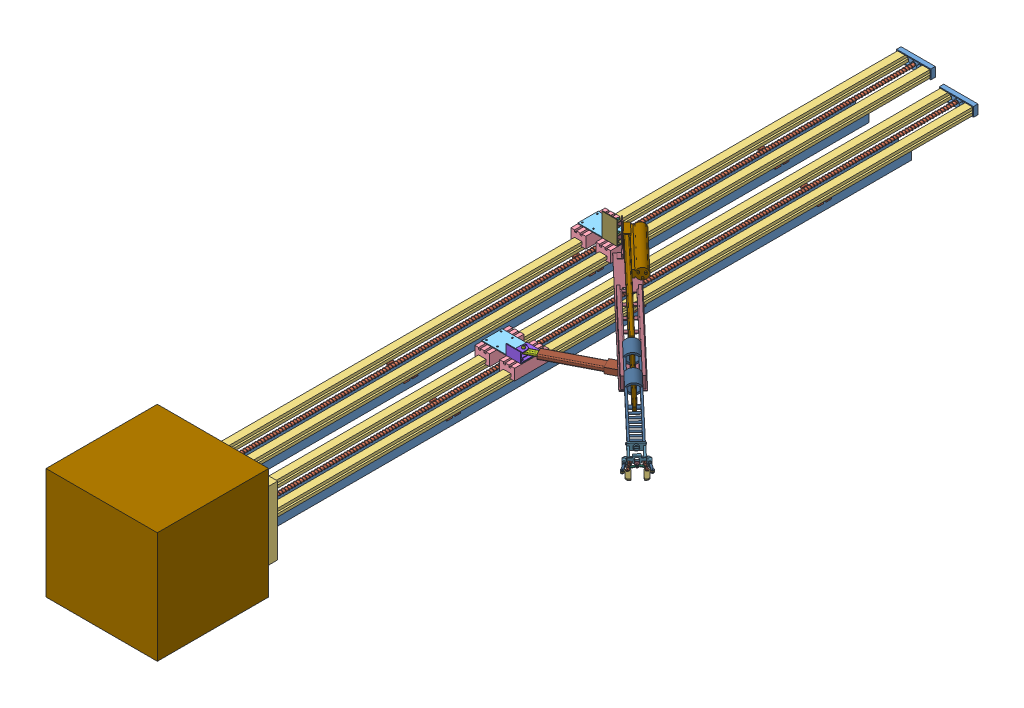
SolidWorks assembly obtox-LIBERO, configuration Default. Lengths in mm.
Overall size (778.48 300 2255.5).
74 component instances, 34 part files, 123 mates.
Components (placement in the parent):
- tapadera de riel-1: tapadera de riel [Default] at (-0.4886 54.6546 45.8092) size (92.3 25.3 12)
- husillo 1900mm-1: husillo 1900mm [Default] at (45.6614 67.3046 1945.8092) x (-0.808521 -0.588468 0) z (0.588468 -0.808521 0) size (10.19 1900.05 10.19)
- tapadera de riel-2: tapadera de riel [Default] at (-115.4886 84.6546 45.8092) size (92.3 25.3 12)
- husillo 1900mm-2: husillo 1900mm [Default] at (-69.3386 97.3046 1945.8092) x (0.990967 -0.134107 0) z (0.134107 0.990967 0) size (10.19 1900.05 10.19)
- guia lineal 2000mm-6: guia lineal 2000mm [Default] at (89.3114 57.1546 1023.3092) x (0 1 0) z (-1 0 0) size (20.3 1950 20.3)
- guia lineal 2000mm-7: guia lineal 2000mm [Default] at (22.3114 57.1546 1023.3092) x (0 1 0) z (-1 0 0) size (20.3 1950 20.3)
- guia lineal 2000mm-8: guia lineal 2000mm [Default] at (-25.6886 87.1546 1023.3092) x (0 1 0) z (-1 0 0) size (20.3 1950 20.3)
- guia lineal 2000mm-9: guia lineal 2000mm [Default] at (-92.6886 87.1546 1023.3092) x (0 1 0) z (-1 0 0) size (20.3 1950 20.3)
- brazo1-1: brazo1 [Default] at (-20.1441 63.0474 912.1315) x (-1 0 0) z (0 0 -1) size (107 44.63 92.2)
  - cojinete-1: cojinete [Default] at (82.6945 46.8572 -15.9576) size (40 30 92.2)
  - cojinete-2: cojinete [Default] at (15.6945 46.8572 -15.9576) size (40 30 92.2)
  - base brazo-1: base brazo [Default] at (49.1945 63.8572 30.1424) x (1 0 0) z (0 -1 0) size (107 55 40.6)
  - tuerca trapezoidal 8-1: tuerca trapezoidal 8 [Default] at (49.1945 34.2572 38.1424) x (0.866025 0.5 0) z (0.5 -0.866025 0) size (22 14.94 22)
- brazo1-2: brazo1 [Default] at (-3.5331 33.0474 1225.8074) size (107 44.63 92.2)
  - cojinete-1: cojinete [Default] at (82.6945 46.8572 -15.9576) size (40 30 92.2)
  - cojinete-2: cojinete [Default] at (15.6945 46.8572 -15.9576) size (40 30 92.2)
  - base brazo-1: base brazo [Default] at (49.1945 63.8572 30.1424) x (1 0 0) z (0 -1 0) size (107 55 40.6)
  - tuerca trapezoidal 8-1: tuerca trapezoidal 8 [Default] at (49.1945 34.2572 38.1424) x (0.866025 0.5 0) z (0.5 -0.866025 0) size (22 14.94 22)
- actuador 1-B-1: actuador 1-B [Default] at (146.7453 121.4046 1238.9625) x (-0.888465 0 0.458945) z (0 -1 0) size (165.5 12 10)
- base actuador 1-2: base actuador 1 [Default] at (59.1614 96.9046 1283.4497) size (40 27 57)
- actuador 1-C-3: actuador 1-C [Default] at (-3.3143 159.4046 907.6709) x (0.725073 0 0.688672) z (0.688672 0 -0.725073) size (384.5 50 48.5)
- deslizante1-1: deslizante1 [Default] at (415.9571 159.4046 1295.5495) x (0.725073 0 0.688672) z (-0.688672 0 0.725073) size (334.5 28.83 40)
- actuador 1-A-5: actuador 1-A [Default] at (253.4869 121.4046 1183.8241) x (-0.888465 0 0.458945) z (0 -1 0) size (184.5 30 15)
- base actuador 3-2: base actuador 3 [Default] at (-55.8386 126.9046 909.4892) size (40 62 29.5)
- Ensamblaje1^obtox-LIBERO-1: Ensamblaje1^obtox-LIBERO [Default] at (400.9916 0 -830.6547) x (0.974334 0 0.225105) z (-0.225105 0 0.974334) size (467.29 65.5 306.35) (virtual)
  - base actuador 2-1: base actuador 2 [Default] at (-2.6233 159.4046 1784.7219) x (0.861487 0 0.507779) z (-0.507779 0 0.861487) size (510 65.5 55)
- servo MG995-1: servo MG995 [Default] at (-79.1886 127.7046 1998.1092) x (1 0 0) z (0 1 0) size (21.2 45.8 54)
- perno2-2: perno2 [Default] at (-21.8386 134.1942 902.4892) x (0.900304 0 -0.435263) z (0 1 0) size (6 6 20)
- perno2-3: perno2 [Default] at (-21.8386 185.6169 902.4892) x (-0.763428 0 0.645893) z (0 -1 0) size (6 6 20)
- perno-3: perno [Default] at (89.6614 124.3697 1268.4497) x (0.731791 0 0.681529) z (0 -1 0) size (8 8 20)
- servo MG995-3: servo MG995 [Default] at (35.8114 97.7046 1998.1092) x (1 0 0) z (0 1 0) size (21.2 45.8 54)
- cople flefible 6x8-2: cople flefible 6x8 [Default] at (45.6614 67.3046 1953.8092) x (0.367009 -0.930217 0) z (0.930217 0.367009 0) size (17.8 25 17.8)
- actuador 1-D-1: actuador 1-D [Default] at (374.5362 159.4046 1245.8643) x (0.725073 0 0.688672) z (-0.688672 0 0.725073) size (368 12 10)
- soporte perfil 40x40x4 mm-2: soporte perfil 40x40x4 mm [Default] at (-49.3386 82.1546 1998.3092) x (-1 0 0) z (0 0 -1) size (40 40 1800)
- soporte L para base-1: soporte L para base [Default] at (-61.8386 17.1546 1998.3092) x (0 1 0) z (0 0 1) size (25 15 25)
- soporte L para base-2: soporte L para base [Default] at (-114.3386 54.6546 1998.3092) size (25 15 25)
- soporte L para base-3: soporte L para base [Default] at (-24.3386 69.6546 1998.3092) x (-1 0 0) z (0 0 1) size (25 15 25)
- soporte L para base-4: soporte L para base [Default] at (-89.3386 62.1546 1438.8092) x (0 1 0) z (1 0 0) size (25 15 25)
- soporte perfil 40x40x4 mm-3: soporte perfil 40x40x4 mm [Default] at (65.6614 52.1546 1998.3092) x (-1 0 0) z (0 0 -1) size (40 40 1800)
- soporte L para base-5: soporte L para base [Default] at (0.6614 24.6546 1998.3092) size (25 15 25)
- soporte L para base-7: soporte L para base [Default] at (53.1614 -12.8454 1998.3092) x (0 1 0) z (0 0 1) size (25 15 25)
- soporte L para base-8: soporte L para base [Default] at (90.6614 39.6546 1998.3092) x (-1 0 0) z (0 0 1) size (25 15 25)
- tapadera de base-1: tapadera de base [Default] at (112.6614 40.3046 1998.3092) x (-1 0 0) z (0 0 -1) size (249 184 44.5)
- tornillo-2: tornillo [Default] at (275.4764 116.9046 1172.4652) x (0.394703 0 -0.918809) z (0 1 0) size (10 11.55 18)
- buje-2: buje [Default] at (275.4764 121.9046 1172.4652) x (0.303677 0 -0.952775) z (0 1 0) size (8 8 10)
- tuerca-2: tuerca [Default] at (275.4764 108.4046 1172.4652) x (-0.848097 0 -0.529841) z (0 1 0) size (10 11.55 5.31)
- cople flefible 6x8-3: cople flefible 6x8 [Default] at (-69.3386 97.3046 1953.8092) x (0.981829 -0.189768 0) z (0.189768 0.981829 0) size (17.8 25 17.8)
- brida para  husillo-3: brida para  husillo [Default] at (-69.3386 97.3046 1928.8092) x (0 -1 0) z (0 0 1) size (45 30 25)
- brida para  husillo-4: brida para  husillo [Default] at (45.6614 67.3046 1928.8092) x (0 -1 0) z (0 0 1) size (45 30 25)
- soporte L para base-9: soporte L para base [Default] at (-49.3386 62.1546 1453.8092) x (0 1 0) z (-1 0 0) size (25 15 25)
- soporte L para base-10: soporte L para base [Default] at (-89.3386 62.1546 938.8092) x (0 1 0) z (1 0 0) size (25 15 25)
- soporte L para base-11: soporte L para base [Default] at (-89.3386 62.1546 438.8092) x (0 1 0) z (1 0 0) size (25 15 25)
- soporte L para base-12: soporte L para base [Default] at (-49.3386 62.1546 953.8092) x (0 1 0) z (-1 0 0) size (25 15 25)
- soporte L para base-13: soporte L para base [Default] at (-49.3386 62.1546 453.8092) x (0 1 0) z (-1 0 0) size (25 15 25)
- soporte L para base-14: soporte L para base [Default] at (0.6614 57.1546 1453.8092) x (1 0 0) z (0 1 0) size (25 15 25)
- soporte L para base-15: soporte L para base [Default] at (65.6614 32.1546 1453.8092) x (0 1 0) z (-1 0 0) size (25 15 25)
- soporte L para base-16: soporte L para base [Default] at (65.6614 32.1546 953.8092) x (0 1 0) z (-1 0 0) size (25 15 25)
- soporte L para base-17: soporte L para base [Default] at (65.6614 32.1546 453.8092) x (0 1 0) z (-1 0 0) size (25 15 25)
- soporte L para base-18: soporte L para base [Default] at (0.6614 57.1546 953.8092) x (1 0 0) z (0 1 0) size (25 15 25)
- soporte L para base-19: soporte L para base [Default] at (0.6614 57.1546 453.8092) x (1 0 0) z (0 1 0) size (25 15 25)
- base-3: base [Default] at (45.6614 67.3046 2001.3092) x (-1 0 0) z (0 0 -1) size (249 184 15)
- soporte-1: soporte [Default] at (-14.1555 78.9736 2001.3092) size (300 300 300)
- pinza-1: pinza [Default] at (541.5071 178.6079 1428.4206) x (0.683645 0.000003 0.729815) z (0.000007 -1 -0.000002) size (126.59 67.98 17)
  - eslabon1-1: eslabon1 [Default] at (16.7384 15.8668 19.3533) x (0.993867 0.110585 0.000003) z (-0.000003 0.000007 1) size (32.5 7.5 7.18)
  - eslabon3-1: eslabon3 [Default] at (16.1548 5.8838 19.3533) x (0.993867 0.110585 0.000003) z (-0.000003 0.000007 1) size (32.5 7.5 7.18)
  - eslabon1-2: eslabon1 [Default] at (13.6225 -37.4322 19.3536) x (0.97421 -0.225641 0.000005) z (-0.000003 0.000007 1) size (32.5 7.5 7.18)
  - clamp-4: clamp [Default] at (29.1618 17.2491 19.4033) x (0.998295 -0.058362 0.000004) z (-0.000003 0.000007 1) size (32.2 19.9 3.4)
  - embolo-1: embolo [Default] at (8.4631 -10.39 23.0534) x (0.058362 0.998295 -0.000007) z (0.000003 -0.000007 -1) size (10 10.75 10)
  - agarradera-amp-1: agarradera-amp [Default] at (-58.5297 18.3293 -31.8016) x (-0.058362 -0.998295 0.000007) z (-0.000003 0.000007 1) size (56.98 73.9 17)
  - clamp-5: clamp [Default] at (25.8001 -40.2528 19.4037) x (0.998295 -0.058362 0.000004) z (0.000003 -0.000007 -1) size (32.2 19.9 3.4)
  - eslabon3-4: eslabon3 [Default] at (14.2061 -27.4493 19.3536) x (0.97421 -0.225641 0.000005) z (0.000003 -0.000007 -1) size (32.5 7.5 7.18)
  - eslabon2-1: eslabon2 [Default] at (8.4631 -10.39 19.5534) x (0.427317 0.904102 -0.000005) z (-0.000003 0.000007 1) size (25.2 7.2 1.5)
  - eslabon2-2: eslabon2 [Default] at (8.4631 -10.39 18.0534) x (0.319055 -0.947736 0.000008) z (-0.000003 0.000007 1) size (25.2 7.2 1.5)
- martillo-2: martillo [Default] at (593.6439 324.9515 1443.0766) x (0.725073 0 0.688672) z (-0.688672 0 0.725073) size (125.98 327.7 54.17) (hidden)
Mates (geometry in assembly coordinates):
- Concéntrica2: concentric aligned: circle of tapadera de riel-1; circle of husillo-1
- Coincidente9: coincident aligned: plane of tapadera de riel-1 through (-0.4886 54.6546 45.8092) normal (0 0 -1); plane of husillo 1900mm-1 through (45.6614 67.3046 45.8092) normal (0 0 -1)
- Coincidente40: coincident: plane of tapadera de riel-1 through (-0.4886 54.6546 45.8092) normal (0 0 -1); plane of tapadera de riel-2 through (-115.4886 84.6546 45.8092) normal (0 0 -1)
- Coincidente45: coincident anti-aligned: plane of tapadera de riel-1 through (-0.4886 57.1546 57.8092) normal (0 1 0); plane of guia lineal 2000mm-6 through (69.0114 57.1546 48.3092) normal (0 -1 0)
- Coincidente46: coincident anti-aligned: plane of tapadera de riel-1 through (89.3114 54.6546 57.8092) normal (-1 0 0); plane of guia lineal 2000mm-6 through (89.3114 57.1546 48.3092) normal (1 0 0)
- Coincidente47: coincident anti-aligned: plane of tapadera de riel-1 through (-0.4886 54.6546 48.3092) normal (0 0 1); plane of guia lineal 2000mm-6 through (89.3114 57.1546 48.3092) normal (0 0 -1)
- Coincidente53: coincident anti-aligned: plane of tapadera de riel-2 through (-115.4886 84.6546 48.3092) normal (0 0 1); plane of guia lineal 2000mm-8 through (-25.6886 87.1546 48.3092) normal (0 0 -1)
- Coincidente59: coincident anti-aligned: plane of tapadera de riel-2 through (-115.4886 87.1546 57.8092) normal (0 1 0); plane of guia lineal 2000mm-9 through (-112.9886 87.1546 48.3092) normal (0 -1 0)
- Coincidente60: coincident anti-aligned: plane of tapadera de riel-2 through (-112.9886 84.6546 57.8092) normal (1 0 0); plane of guia lineal 2000mm-9 through (-112.9886 94.8046 48.3092) normal (-1 0 0)
- Concéntrica4: concentric anti-aligned: circle of tapadera de riel-2; circle of brazo1-1/tuerca trapezoidal-1
- Paralelo1: parallel aligned: plane of guia lineal 2000mm-8 through (-25.6886 107.4546 48.3092) normal (0 1 0); plane of brazo1-1/cojinete-2 through (-15.8386 124.9046 835.8892) normal (0 1 0)
- Concéntrica5: concentric aligned: circle of husillo-1; circle of brazo1-2/tuerca trapezoidal-1
- Paralelo2: parallel aligned: plane of guia lineal 2000mm-6 through (89.3114 77.4546 48.3092) normal (0 1 0); plane of brazo1-2/base brazo-1 through (45.6614 96.9046 1255.9497) normal (0 1 0)
- Concéntrica6: concentric anti-aligned: circle of brazo1-2/base brazo-1; circle of base actuador 1-1
- Concéntrica7: concentric anti-aligned: circle of brazo1-2/base brazo-1; circle of base actuador 1-1
- Concéntrica8: concentric anti-aligned: circle of brazo1-2/base brazo-1; circle of base actuador 1-1
- Coincidente61: coincident anti-aligned: plane of brazo1-2/base brazo-1 through (45.6614 96.9046 1255.9497) normal (0 1 0); plane of base actuador 1-2 through (59.1614 96.9046 1283.4497) normal (0 -1 0)
- Concéntrica9: concentric anti-aligned: circle of actuador 1-B-1; circle of base actuador 1-1
- Coincidente64: coincident anti-aligned: plane of actuador 1-B-1 through (146.7453 118.9046 1238.9625) normal (0 1 0); plane of base actuador 1-2 through (89.6614 118.9046 1268.4497) normal (0 -1 0)
- Paralelo4: parallel aligned: plane of tapadera de riel-2 through (-115.4886 109.9546 57.8092) normal (0 1 0); plane of actuador 1-C-3 through (-6.5793 174.4046 883.8822) normal (0 1 0)
- Paralelo5: parallel aligned: plane of actuador 1-C-3 through (-6.5793 174.4046 883.8822) normal (0 1 0); plane of deslizante1-1 through (428.0088 163.9046 1282.8607) normal (0 1 0)
- Concéntrica16: concentric anti-aligned: circle of brazo1-1/base brazo-1; circle of base actuador 3-2
- Concéntrica17: concentric anti-aligned: circle of brazo1-1/base brazo-1; circle of base actuador 3-2
- Coincidente83: coincident anti-aligned: plane of brazo1-1/base brazo-1 through (-69.3386 126.9046 881.9892) normal (0 1 0); plane of base actuador 3-2 through (-55.8386 126.9046 909.4892) normal (0 -1 0)
- Concéntrica31: concentric anti-aligned: circle of perno2-2; circle of base actuador 3-2
- Concéntrica32: concentric anti-aligned: circle of base actuador 3-2; circle of perno2-3
- Concéntrica34: concentric anti-aligned: circle of base actuador 1-2; circle of perno-3
- Coincidente91: coincident aligned: plane of servo MG995-1 through (-73.9886 83.6546 1965.7092) normal (0 0 -1); plane of servo MG995-3 through (41.0114 101.7546 1965.7092) normal (0 0 -1)
- Concéntrica37: concentric anti-aligned: circle of servo MG995-3; circle of cople-2
- Coincidente96: coincident anti-aligned: plane of actuador 1-C-3 through (20.4486 165.4046 917.1387) normal (0 -1 0); plane of actuador 1-D-1 through (404.9005 165.4046 1291.9438) normal (0 1 0)
- Coincidente97: coincident anti-aligned: plane of actuador 1-C-3 through (22.5146 162.4046 914.9635) normal (-0.688672 0 0.725073); plane of actuador 1-D-1 through (372.8145 159.4046 1247.677) normal (0.688672 0 -0.725073)
- Concéntrica40: concentric anti-aligned: cylinder of deslizante1-1 through (407.3487 159.4046 1304.6129) axis (0.688672 0 -0.725073) radius 4.5; circle of actuador 1-D-1
- Coincidente101: coincident anti-aligned: plane of soporte perfil 40x40x4 mm-2 through (-89.3386 42.1546 198.3092) normal (0 -1 0); plane of soporte L para base-1 through (-76.8386 42.1546 1996.3092) normal (0 1 0)
- Concéntrica41: concentric aligned: circle of soporte perfil 40x40x4 mm-2; circle of soporte L para base-1
- Concéntrica42: concentric anti-aligned: circle of soporte perfil 40x40x4 mm-2; circle of soporte L para base-2
- Coincidente102: coincident anti-aligned: plane of soporte perfil 40x40x4 mm-2 through (-89.3386 82.1546 198.3092) normal (-1 0 0); plane of soporte L para base-2 through (-89.3386 69.6546 1996.3092) normal (1 0 0)
- Concéntrica43: concentric aligned: circle of soporte perfil 40x40x4 mm-2; circle of soporte L para base-3
- Coincidente104: coincident anti-aligned: plane of soporte perfil 40x40x4 mm-2 through (-49.3386 42.1546 198.3092) normal (1 0 0); plane of soporte L para base-3 through (-49.3386 54.6546 1996.3092) normal (-1 0 0)
- Coincidente106: coincident anti-aligned: plane of soporte perfil 40x40x4 mm-2 through (-89.3386 82.1546 198.3092) normal (-1 0 0); plane of soporte L para base-4 through (-89.3386 62.1546 1453.8092) normal (1 0 0)
- Coincidente108: coincident anti-aligned: plane of guia lineal 2000mm-9 through (-112.9886 87.1546 48.3092) normal (0 -1 0); plane of soporte L para base-4 through (-91.3386 87.1546 1453.8092) normal (0 1 0)
- Concéntrica45: concentric aligned: circle of husillo 1900mm-1; circle of cople flefible 6x8-2
- Distancia1: distance = 3.35 mm anti-aligned: plane of soporte perfil 40x40x4 mm-2 through (-49.3386 42.1546 198.3092) normal (1 0 0); plane of guia lineal 2000mm-8 through (-45.9886 94.8046 48.3092) normal (-1 0 0)
- Distancia2: distance = 3.35 mm anti-aligned: plane of soporte perfil 40x40x4 mm-3 through (25.6614 52.1546 198.3092) normal (-1 0 0); plane of guia lineal 2000mm-7 through (22.3114 57.1546 48.3092) normal (1 0 0)
- Concéntrica48: concentric anti-aligned: circle of soporte perfil 40x40x4 mm-3; circle of soporte L para base-5
- Concéntrica51: concentric aligned: circle of soporte perfil 40x40x4 mm-3; circle of soporte L para base-8
- Coincidente116: coincident anti-aligned: plane of soporte perfil 40x40x4 mm-3 through (65.6614 12.1546 198.3092) normal (1 0 0); plane of soporte L para base-8 through (65.6614 24.6546 1996.3092) normal (-1 0 0)
- Distancia3: distance = 20 mm aligned: plane of soporte perfil 40x40x4 mm-2 through (-89.3386 42.1546 198.3092) normal (0 -1 0); plane of soporte L para base-4 through (-92.3386 62.1546 1453.8092) normal (0 -1 0)
- Coincidente118: coincident anti-aligned: plane of soporte perfil 40x40x4 mm-3 through (25.6614 12.1546 198.3092) normal (0 -1 0); plane of soporte L para base-7 through (38.1614 12.1546 1996.3092) normal (0 1 0)
- Concéntrica59: concentric aligned: circle of buje-2; circle of tuerca-2
- Tornillo3: screw = 1 mm aligned: cylinder of husillo 1900mm-1 through (45.6614 67.3046 45.8092) axis (0 0 1) radius 4; cylinder of brazo1-2/tuerca trapezoidal 8-1 through (45.6614 67.3046 1250.4497) axis (0 0 1) radius 4.5
- Coincidente126: coincident anti-aligned: plane of cople flefible 6x8-2 through (48.9278 59.0257 1953.8092) normal (0 0 1); plane of tapadera de base-1 through (112.6614 40.3046 1953.8092) normal (0 0 -1)
- Concéntrica61: concentric anti-aligned: circle of tapadera de base-1; circle of cople flefible 6x8-3
- Coincidente127: coincident aligned: plane of cople flefible 6x8-2 through (45.6614 67.3046 1928.8092) normal (0 0 -1); plane of cople flefible 6x8-3 through (-69.3386 97.3046 1928.8092) normal (0 0 -1)
- Concéntrica62: concentric aligned: circle of cople flefible 6x8-3; circle of brida para  husillo-3
- Paralelo7: parallel anti-aligned: plane of tapadera de base-1 through (-136.3386 40.3046 1953.8092) normal (-1 0 0); plane of brida para  husillo-3 through (-54.3386 109.8046 1953.8092) normal (1 0 0)
- Paralelo8: parallel aligned: plane of servo MG995-1 through (-79.1886 127.7046 1998.1092) normal (-1 0 0); plane of brida para  husillo-3 through (-84.3386 119.8046 1953.8092) normal (-1 0 0)
- Paralelo9: parallel aligned: plane of servo MG995-1 through (-79.1886 127.7046 1998.1092) normal (-1 0 0); plane of servo MG995-3 through (35.8114 97.7046 1998.1092) normal (-1 0 0)
- Coincidente129: coincident anti-aligned: plane of tapadera de base-1 through (112.6614 40.3046 1953.8092) normal (0 0 -1); plane of brida para  husillo-3 through (-69.3386 97.3046 1953.8092) normal (0 0 1)
- Concéntrica63: concentric aligned: circle of cople flefible 6x8-2; circle of brida para  husillo-4
- Coincidente130: coincident aligned: plane of brida para  husillo-3 through (-69.3386 97.3046 1928.8092) normal (0 0 -1); plane of brida para  husillo-4 through (45.6614 67.3046 1928.8092) normal (0 0 -1)
- Paralelo10: parallel aligned: plane of brida para  husillo-3 through (-84.3386 119.8046 1953.8092) normal (-1 0 0); plane of brida para  husillo-4 through (30.6614 89.8046 1953.8092) normal (-1 0 0)
- Distancia5: distance = 500 mm anti-aligned: plane of soporte L para base-4 through (-91.3386 85.1546 1453.8092) normal (0 0 1); plane of tapadera de base-1 through (112.6614 40.3046 1953.8092) normal (0 0 -1)
- Coincidente131: coincident anti-aligned: plane of soporte perfil 40x40x4 mm-2 through (-49.3386 42.1546 198.3092) normal (1 0 0); plane of soporte L para base-9 through (-49.3386 62.1546 1438.8092) normal (-1 0 0)
- Coincidente132: coincident aligned: plane of soporte L para base-4 through (-91.3386 85.1546 1438.8092) normal (0 0 -1); plane of soporte L para base-9 through (-47.3386 85.1546 1438.8092) normal (0 0 -1)
- Coincidente133: coincident aligned: plane of soporte L para base-4 through (-92.3386 62.1546 1453.8092) normal (0 -1 0); plane of soporte L para base-9 through (-46.3386 62.1546 1438.8092) normal (0 -1 0)
- Coincidente134: coincident aligned: plane of soporte L para base-9 through (-47.3386 85.1546 1438.8092) normal (0 0 -1); plane of soporte L para base-14 through (23.6614 55.1546 1438.8092) normal (0 0 -1)
- Coincidente135: coincident anti-aligned: plane of soporte perfil 40x40x4 mm-3 through (25.6614 52.1546 198.3092) normal (-1 0 0); plane of soporte L para base-14 through (25.6614 55.1546 1438.8092) normal (1 0 0)
- Coincidente136: coincident anti-aligned: plane of guia lineal 2000mm-7 through (2.0114 57.1546 48.3092) normal (0 -1 0); plane of soporte L para base-14 through (0.6614 57.1546 1438.8092) normal (0 1 0)
- Coincidente137: coincident anti-aligned: plane of soporte perfil 40x40x4 mm-3 through (65.6614 12.1546 198.3092) normal (1 0 0); plane of soporte L para base-15 through (65.6614 32.1546 1438.8092) normal (-1 0 0)
- Coincidente138: coincident anti-aligned: plane of guia lineal 2000mm-6 through (69.0114 57.1546 48.3092) normal (0 -1 0); plane of soporte L para base-15 through (67.6614 57.1546 1438.8092) normal (0 1 0)
- Coincidente139: coincident aligned: plane of soporte L para base-14 through (23.6614 55.1546 1438.8092) normal (0 0 -1); plane of soporte L para base-15 through (67.6614 55.1546 1438.8092) normal (0 0 -1)
- Coincidente140: coincident anti-aligned: plane of actuador 1-C-3; plane of actuador 1-D-1
- Concéntrica64: concentric aligned: circle of servo MG995-1; circle of cople flefible 6x8-3
- Coincidente141: coincident anti-aligned: plane of servo MG995-1 through (-69.3386 97.3046 1955.8092) normal (0 0 -1); plane of tapadera de base-1 through (112.6614 40.3046 1955.8092) normal (0 0 1)
- Concéntrica66: concentric anti-aligned: circle of tapadera de base-1; circle of brida para  husillo-4
- Coincidente142: coincident aligned: plane of tapadera de base-1 through (-136.3386 40.3046 1953.8092) normal (-1 0 0); plane of base-3 through (-136.3386 70.3046 1998.3092) normal (-1 0 0)
- Coincidente143: coincident aligned: plane of tapadera de base-1 through (112.6614 164.3046 2254.4361) normal (0 1 0); plane of base-3 through (112.6614 164.3046 2257.4361) normal (0 1 0)
- Coincidente144: coincident anti-aligned: plane of soporte L para base-1 through (-76.8386 17.1546 1998.3092) normal (0 0 1); plane of base-3 through (-69.3386 97.3046 1998.3092) normal (0 0 -1)
- Coincidente145: coincident anti-aligned: plane of tapadera de base-1 through (112.6614 40.3046 1998.3092) normal (0 0 1); plane of base-3 through (-69.3386 97.3046 1998.3092) normal (0 0 -1)
- Coincidente146: coincident anti-aligned: plane of tapadera de riel-2 through (-115.4886 107.4546 57.8092) normal (0 -1 0); plane of guia lineal 2000mm-8 through (-25.6886 107.4546 48.3092) normal (0 1 0)
- Coincidente147: coincident anti-aligned: plane of tapadera de riel-2 through (-25.6886 84.6546 57.8092) normal (-1 0 0); plane of guia lineal 2000mm-8 through (-25.6886 87.1546 48.3092) normal (1 0 0)
- Distancia8: distance = 3.35 mm anti-aligned: plane of guia lineal 2000mm-6 through (69.0114 64.8046 48.3092) normal (-1 0 0); plane of soporte perfil 40x40x4 mm-3 through (65.6614 12.1546 198.3092) normal (1 0 0)
- Coincidente149: coincident anti-aligned: plane of soporte L para base-7 through (38.1614 -12.8454 1998.3092) normal (0 0 1); plane of base-3 through (-69.3386 97.3046 1998.3092) normal (0 0 -1)
- Coincidente150: coincident aligned: circle of soporte L para base-5; circle of base-3
- Coincidente152: coincident anti-aligned: plane of soporte L para base-8 through (90.6614 24.6546 1998.3092) normal (0 0 1); plane of base-3 through (-69.3386 97.3046 1998.3092) normal (0 0 -1)
- Concéntrica67: concentric aligned: circle of soporte perfil 40x40x4 mm-3; circle of soporte L para base-7
- Coincidente153: coincident anti-aligned: plane of soporte L para base-3 through (-24.3386 54.6546 1998.3092) normal (0 0 1); plane of base-3 through (-69.3386 97.3046 1998.3092) normal (0 0 -1)
- Coincidente154: coincident aligned: circle of soporte L para base-2; plane of base-3 through (-69.3386 97.3046 1998.3092) normal (0 0 -1)
- Coincidente156: coincident aligned: plane of soporte L para base-17 through (68.6614 32.1546 438.8092) normal (0 -1 0); plane of soporte L para base-19 through (25.6614 32.1546 438.8092) normal (0 -1 0)
- Coincidente158: coincident anti-aligned: plane of base-3 through (-69.3386 97.3046 2001.3092) normal (0 0 1); plane of soporte-1 through (-14.1555 78.9736 2001.3092) normal (0 0 -1)
- Concéntrica69: concentric anti-aligned: circle of actuador 1-A-5; circle of buje-2
- Coincidente161: coincident anti-aligned: plane of actuador 1-B-1 through (146.7453 108.9046 1238.9625) normal (0 -1 0); plane of actuador 1-A-5 through (233.7627 108.9046 1197.3895) normal (0 1 0)
- Concéntrica72: concentric aligned: circle of tornillo-2; circle of buje-2
- Coincidente162: coincident anti-aligned: plane of actuador 1-A-5 through (282.2134 113.4046 1174.6128) normal (0 -1 0); plane of tuerca-2 through (275.4764 113.4046 1172.4652) normal (0 1 0)
- Distancia límite1: limit distance = 186.8735 mm anti-aligned: plane of actuador 1-D-1 through (153.1908 156.4046 1048.7335) normal (-0.725073 0 -0.688672); plane of actuador 1-C-3 through (17.6939 162.4046 920.039) normal (0.725073 0 0.688672)
- Distancia límite3: limit distance = 2.6416 mm anti-aligned: plane of actuador 1-B-1 through (231.4157 115.9046 1198.6018) normal (0.888465 0 -0.458945); plane of actuador 1-A-5 through (233.7627 115.9046 1197.3895) normal (-0.888465 0 0.458945)
- Concéntrica74: concentric aligned: circle of tapadera de riel-2; circle of husillo 1900mm-2
- Coincidente165: coincident aligned: plane of tapadera de riel-2 through (-115.4886 84.6546 45.8092) normal (0 0 -1); plane of husillo 1900mm-2 through (-69.3386 97.3046 45.8092) normal (0 0 -1)
- Tornillo4: screw = 8 mm anti-aligned: cylinder of husillo 1900mm-2 through (-69.3386 97.3046 45.8092) axis (0 0 1) radius 4; cylinder of brazo1-1/tuerca trapezoidal 8-1 through (-69.3386 97.3046 887.4892) axis (0 0 -1) radius 4.5
- Concéntrica75: concentric anti-aligned: circle of actuador 1-C-3; circle of Ensamblaje1^obtox-1/base actuador 2-1
- Concéntrica76: concentric anti-aligned: circle of actuador 1-C-3; circle of Ensamblaje1^obtox-1/base actuador 2-1
- Coincidente166: coincident anti-aligned: plane of actuador 1-C-3; plane of Ensamblaje1^obtox-1/base actuador 2-1
- Concéntrica77: concentric anti-aligned: circle of base actuador 3-2; circle of Ensamblaje1^obtox-1/base actuador 2-1
- Coincidente167: coincident anti-aligned: plane of base actuador 3-2 through (-21.8386 138.9046 1712.3707) normal (0 1 0); plane of Ensamblaje1^obtox-1/base actuador 2-1 through (-21.8386 138.9046 1712.3707) normal (0 -1 0)
- Coincidente168: coincident aligned: plane of Ensamblaje1^obtox-1/base actuador 2-1 through (-3.9532 131.9046 1719.4498) normal (0 1 0); plane of buje-2 through (245.8048 131.9046 2011.7872) normal (0 1 0)
- Coincidente169: coincident anti-aligned: plane of Ensamblaje1^obtox-1/base actuador 2-1 through (-3.9532 131.9046 1719.4498) normal (0 1 0); plane of tornillo-2 through (245.8048 131.9046 2011.7872) normal (0 -1 0)
- Concéntrica78: concentric anti-aligned: circle of actuador 1-C-3; circle of Ensamblaje1^obtox-1/base actuador 2-1
- Coincidente170: coincident anti-aligned: plane of deslizante1-1; plane of Ensamblaje1^obtox-1/base actuador 2-1
- Concéntrica79: concentric anti-aligned: circle of actuador 1-A-5; circle of Ensamblaje1^obtox-1/base actuador 2-1
- Concéntrica81: concentric anti-aligned: circle of base actuador 3-2; circle of Ensamblaje1^obtox-1/base actuador 2-1
- Coincidente171: coincident anti-aligned: plane of base actuador 3-2 through (-21.8386 179.9046 902.4892) normal (0 -1 0); plane of Ensamblaje1^obtox-1/base actuador 2-1 through (-21.8386 179.9046 902.4892) normal (0 1 0)
- Coincidente172: coincident anti-aligned: plane of actuador 1-C-3 through (-3.3143 159.4046 907.6709) normal (-0.688672 0 0.725073); plane of Ensamblaje1^obtox-1/base actuador 2-1 through (-3.3143 159.4046 907.6709) normal (0.688672 0 -0.725073)
- Coincidente173: coincident anti-aligned: plane of deslizante1-1 through (428.0088 159.4046 1282.8607) normal (0.688672 0 -0.725073); plane of Ensamblaje1^obtox-1/base actuador 2-1 through (357.2247 163.9046 1215.6302) normal (-0.688672 0 0.725073)
- Coincidente174: coincident aligned: plane of deslizante1-1 through (428.0088 163.9046 1282.8607) normal (0 1 0); plane of Ensamblaje1^obtox-1/base actuador 2-1 through (-3.3143 163.9046 907.6709) normal (0 1 0)
- Concéntrica82: concentric anti-aligned: circle of buje-2; circle of Ensamblaje1^obtox-1/base actuador 2-1
- Concéntrica83: concentric anti-aligned: circle of actuador 1-C-3; circle of Ensamblaje1^obtox-1/base actuador 2-1
- Paralelo11: parallel aligned: plane of deslizante1-1 through (428.0088 163.9046 1282.8607) normal (0 1 0); plane of pinza-1/agarradera-amp-1 through (533.8863 161.9046 1441.472) normal (0 1 0)
- Coincidente175: coincident anti-aligned: plane of deslizante1-1 through (407.3487 159.4046 1304.6129) normal (0.688672 0 -0.725073); plane of pinza-1/agarradera-amp-1 through (494.3575 159.4046 1387.2535) normal (-0.688672 0 0.725073)
- Concéntrica84: concentric aligned: circle of deslizante1-1; circle of pinza-1/agarradera-amp-1
- Coincidente178: coincident anti-aligned: plane of pinza-1/clamp-4 through (580.8174 193.7151 1469.3728) normal (0.688672 0 -0.725073); plane of martillo-2 through (581.2937 209.9515 1469.8252) normal (-0.688672 0 0.725073)
- Bloquear1: lock: unknown of pinza-1/clamp-4; unknown of martillo-2
- Bloquear2: lock: unknown of pinza-1/clamp-4; unknown of martillo-2
- Coincidente179: coincident anti-aligned: plane of actuador 1-B-1 through (85.7516 108.9046 1277.2226) normal (0.458945 0 0.888465); plane of actuador 1-A-5 through (235.1395 111.9046 1200.0548) normal (-0.458945 0 -0.888465)
